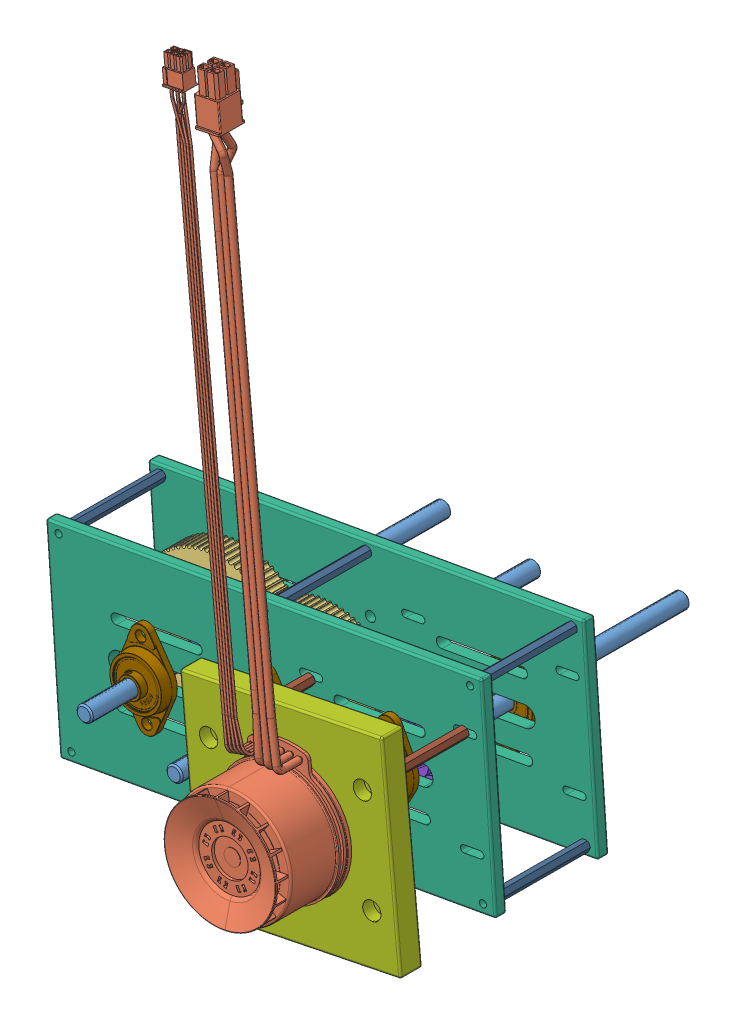
SolidWorks assembly Assembly, configuration Default. Lengths in mm.
Overall size (235.9 403.12 260.01).
25 component instances, 11 part files, 48 mates.
Components (placement in the parent):
- 1265K64_Rotary Shaft-1: 1265K64_Rotary Shaft [1265K64] at (277.2375 -256.7414 10.4805) x (-0.834942 -0.544047 0.082971) z (0.05862 0.061986 0.996354) size (8 8 200)
- 1265K64_Rotary Shaft-2: 1265K64_Rotary Shaft [1265K64] at (218.9474 -262.2229 29.581) x (0.998279 -0.00182 -0.05862) z (0.05862 0.061986 0.996354) size (8 8 200)
- 1265K64_Rotary Shaft-3: 1265K64_Rotary Shaft [1265K64] at (159.0131 -271.6943 16.4934) x (0.995771 0.067098 -0.06276) z (0.05862 0.061986 0.996354) size (8 8 200)
- EC60fl-200W-V2.stp-1: EC60fl-200W-V2.stp [Default] at (282.4403 -251.2399 98.9109) x (0.05862 0.061986 0.996354) z (0.986782 0.14745 -0.067231) size (68.19 353.93 60)
- 80 tooth pulley.stp-1: 80 tooth pulley.stp [Default] at (220.6003 -260.4751 57.675) x (0.997636 0.032205 -0.060699) z (0.05862 0.061986 0.996354) size (75.56 75.56 22.21)
- 80 tooth pulley.stp-2: 80 tooth pulley.stp [Default] at (160.6699 -269.9423 44.6536) x (0.983509 -0.174648 -0.046999) z (0.05862 0.061986 0.996354) size (75.56 75.56 22.21)
- 2463K28_Clamping Precision Flexible Shaft Coupling-1: 2463K28_Clamping Precision Flexible Shaft Coupling [2463K28] at (282.4471 -251.2327 99.0265) x (-0.5684 -0.818416 0.084358) z (0.05862 0.061986 0.996354) size (26.29 26.14 30)
- 94630A112_Steel Oversized Washer-1: 94630A112_Steel Oversized Washer [94630A112] at (219.6037 -261.5289 40.737) x (0.842889 -0.537845 -0.01613) z (0.05862 0.061986 0.996354) size (23 23 4.3)
- Shaft_and_Bearing_plate-1: Shaft_and_Bearing_plate [Default] at (221.2998 -259.7354 69.5646) x (0.99004 0.124365 -0.065986) z (0.128002 -0.990298 0.054079) size (215 6 100)
- Shaft_and_Bearing_plate-2: Shaft_and_Bearing_plate [Default] at (217.9702 -263.2563 12.9717) x (0.99004 0.124365 -0.065986) z (0.128002 -0.990298 0.054079) size (215 6 100)
- motor_plate-1: motor_plate [Default] at (283.4427 -250.1799 115.9486) x (-0.986782 -0.14745 0.067231) z (-0.151079 0.987125 -0.052524) size (100 12 100)
- 30toothpulley.stp-1: 30toothpulley.stp [Default] at (279.8164 -254.0145 54.3129) x (0.779271 0.620967 -0.084481) z (0.05862 0.061986 0.996354) size (31.8 31.8 20.6)
- 30toothpulley.stp-2: 30toothpulley.stp [Default] at (218.8358 -262.3409 27.6848) x (-0.996812 -0.050484 0.061788) z (-0.05862 -0.061986 -0.996354) size (31.8 31.8 20.6)
- KFL08 - Mancal Flange oval Ø8.stp-1: KFL08 - Mancal Flange oval Ø8.stp [Default] at (217.9702 -263.2563 12.9717) x (0.128002 -0.990298 0.054079) z (0.99004 0.124365 -0.065986) size (47.88 11.35 28.12)
- KFL08 - Mancal Flange oval Ø8.stp-2: KFL08 - Mancal Flange oval Ø8.stp [Default] at (159.0407 -271.6651 16.9619) x (0.043052 -0.997299 0.059512) z (0.997352 0.039406 -0.061131) size (47.88 11.35 28.12)
- KFL08 - Mancal Flange oval Ø8.stp-3: KFL08 - Mancal Flange oval Ø8.stp [Default] at (162.722 -267.7724 79.533) x (0.143739 -0.988194 0.053022) z (-0.987878 -0.140107 0.066838) size (47.88 11.35 28.12)
- KFL08 - Mancal Flange oval Ø8.stp-4: KFL08 - Mancal Flange oval Ø8.stp [Default] at (221.6515 -259.3635 75.5427) x (-0.128002 0.990298 -0.054079) z (0.99004 0.124365 -0.065986) size (47.88 11.35 28.12)
- KFL08 - Mancal Flange oval Ø8.stp-5: KFL08 - Mancal Flange oval Ø8.stp [Default] at (277.1557 -256.828 9.0896) x (-0.089563 0.994372 -0.056594) z (-0.994255 -0.085919 0.063842) size (47.88 11.35 28.12)
- KFL08 - Mancal Flange oval Ø8.stp-6: KFL08 - Mancal Flange oval Ø8.stp [Default] at (280.837 -252.9352 71.6606) x (-0.024433 0.99786 -0.060643) z (0.997981 0.020789 -0.06001) size (47.88 11.35 28.12)
- 91115A824_Female Threaded Hex Standoff 2in-1: 91115A824_Female Threaded Hex Standoff 2in [91115A824] at (314.4758 -203.6283 35.099) x (0.981398 0.179196 -0.068889) z (0.05862 0.061986 0.996354) size (4.76 5.5 51.24)
- 91115A824_Female Threaded Hex Standoff 2in-2: 91115A824_Female Threaded Hex Standoff 2in [91115A824] at (326.124 -293.7454 40.0202) x (-0.91308 0.40679 0.028413) z (-0.05862 -0.061986 -0.996354) size (4.76 5.5 51.24)
- 91115A824_Female Threaded Hex Standoff 2in-3: 91115A824_Female Threaded Hex Standoff 2in [91115A824] at (213.9868 -216.2513 41.7966) x (0.988326 0.136991 -0.066671) z (-0.05862 -0.061986 -0.996354) size (4.76 5.5 51.24)
- 91115A824_Female Threaded Hex Standoff 2in-4: 91115A824_Female Threaded Hex Standoff 2in [91115A824] at (113.4977 -228.8743 48.4942) x (0.263743 -0.963569 0.044429) z (-0.05862 -0.061986 -0.996354) size (4.76 5.5 51.24)
- 91115A822_Female Threaded Hex Standoff 1 and 3_4ths-1: 91115A822_Female Threaded Hex Standoff 1 and 3_4ths [91115A822] at (315.8606 -221.2764 89.9367) x (0.90677 0.414135 -0.079114) z (0.05862 0.061986 0.996354) size (4.76 5.5 44.89)
- 91115A822_Female Threaded Hex Standoff 1 and 3_4ths-2: 91115A822_Female Threaded Hex Standoff 1 and 3_4ths [91115A822] at (240.8652 -232.4825 95.0463) x (0.90677 0.414135 -0.079114) z (0.05862 0.061986 0.996354) size (4.76 5.5 44.89)
Mates (geometry in assembly coordinates):
- Concentric2: concentric aligned: cylinder of 1265K64_Rotary Shaft-2 through (224.8094 -256.0243 129.2164) axis (-0.05862 -0.061986 -0.996354) radius 4; cylinder of 80 tooth pulley.stp-1 through (221.185 -259.8568 67.6137) axis (-0.05862 -0.061986 -0.996354) radius 4
- Concentric3: concentric aligned: cylinder of 1265K64_Rotary Shaft-3 through (164.8752 -265.4956 116.1288) axis (-0.05862 -0.061986 -0.996354) radius 4; cylinder of 80 tooth pulley.stp-2 through (161.2547 -269.324 54.5922) axis (-0.05862 -0.061986 -0.996354) radius 4
- Concentric4: concentric aligned: cylinder of 1265K64_Rotary Shaft-2 through (224.8094 -256.0243 129.2164) axis (-0.05862 -0.061986 -0.996354) radius 4; cylinder of 94630A112_Steel Oversized Washer-1 through (219.8558 -261.2623 45.0213) axis (-0.05862 -0.061986 -0.996354) radius 4.2
- Concentric22: concentric aligned: cylinder of 1265K64_Rotary Shaft-2 through (224.8094 -256.0243 129.2164) axis (-0.05862 -0.061986 -0.996354) radius 4; cylinder of Shaft_and_Bearing_plate-2 through (218.3219 -262.8843 18.9498) axis (-0.05862 -0.061986 -0.996354) radius 5
- Coincident9: coincident anti-aligned: plane of 80 tooth pulley.stp-1 through (219.8558 -261.2623 45.0213) normal (-0.05862 -0.061986 -0.996354); plane of 94630A112_Steel Oversized Washer-1 through (219.8558 -261.2623 45.0213) normal (0.05862 0.061986 0.996354)
- Tangent8: tangent anti-aligned: cylinder of 1265K64_Rotary Shaft-3 through (164.8752 -265.4956 116.1288) axis (-0.05862 -0.061986 -0.996354) radius 4; plane of Shaft_and_Bearing_plate-1 through (187.6401 -268.6678 78.1226) normal (-0.128002 0.990298 -0.054079)
- Parallel3: parallel aligned: cylinder of 1265K64_Rotary Shaft-2 through (224.8094 -256.0243 129.2164) axis (-0.05862 -0.061986 -0.996354) radius 4; cylinder of 1265K64_Rotary Shaft-3 through (164.8752 -265.4956 116.1288) axis (-0.05862 -0.061986 -0.996354) radius 4
- Tangent9: tangent anti-aligned: cylinder of 1265K64_Rotary Shaft-1 through (283.0995 -250.5428 110.1159) axis (-0.05862 -0.061986 -0.996354) radius 4; plane of Shaft_and_Bearing_plate-2 through (253.6133 -263.4831 16.9107) normal (-0.128002 0.990298 -0.054079)
- Parallel4: parallel aligned: cylinder of 1265K64_Rotary Shaft-1 through (283.0995 -250.5428 110.1159) axis (-0.05862 -0.061986 -0.996354) radius 4; cylinder of 1265K64_Rotary Shaft-2 through (224.8094 -256.0243 129.2164) axis (-0.05862 -0.061986 -0.996354) radius 4
- Distance3: distance = 59.66 mm: cylinder of 1265K64_Rotary Shaft-2 through (224.8094 -256.0243 129.2164) axis (-0.05862 -0.061986 -0.996354) radius 4; cylinder of 1265K64_Rotary Shaft-1 through (283.0995 -250.5428 110.1159) axis (-0.05862 -0.061986 -0.996354) radius 4
- Distance4: distance = 59.66 mm: cylinder of 1265K64_Rotary Shaft-3 through (164.8752 -265.4956 116.1288) axis (-0.05862 -0.061986 -0.996354) radius 4; cylinder of 1265K64_Rotary Shaft-2 through (224.8094 -256.0243 129.2164) axis (-0.05862 -0.061986 -0.996354) radius 4
- Concentric34: concentric aligned: cylinder of 1265K64_Rotary Shaft-1 through (283.0995 -250.5428 110.1159) axis (-0.05862 -0.061986 -0.996354) radius 4; cylinder of motor_plate-1 through (283.7944 -249.808 121.9267) axis (-0.05862 -0.061986 -0.996354) radius 13.5
- Concentric35: concentric anti-aligned: cylinder of 1265K64_Rotary Shaft-1 through (283.0995 -250.5428 110.1159) axis (-0.05862 -0.061986 -0.996354) radius 4; cylinder of EC60fl-200W-V2.stp-1 through (282.2606 -251.4299 95.8571) axis (0.05862 0.061986 0.996354) radius 4
- Concentric36: concentric aligned: cylinder of EC60fl-200W-V2.stp-1 through (264.2888 -241.4217 130.9743) axis (-0.05862 -0.061986 -0.996354) radius 1.65; cylinder of motor_plate-1 through (263.7969 -241.9419 122.6139) axis (-0.05862 -0.061986 -0.996354) radius 2.65
- Coincident20: coincident anti-aligned: plane of EC60fl-200W-V2.stp-1 through (283.7944 -249.808 121.9267) normal (-0.05862 -0.061986 -0.996354); plane of motor_plate-1 through (283.7944 -249.808 121.9267) normal (0.05862 0.061986 0.996354)
- Concentric38: concentric anti-aligned: cylinder of EC60fl-200W-V2.stp-1 through (282.2606 -251.4299 95.8571) axis (0.05862 0.061986 0.996354) radius 4; cylinder of 2463K28_Clamping Precision Flexible Shaft Coupling-1 through (283.3264 -250.3029 113.9718) axis (-0.05862 -0.061986 -0.996354) radius 4
- Concentric44: concentric anti-aligned: cylinder of 1265K64_Rotary Shaft-1 through (283.0995 -250.5428 110.1159) axis (-0.05862 -0.061986 -0.996354) radius 4; cylinder of 30toothpulley.stp-1 through (278.3852 -255.5278 29.9882) axis (0.05862 0.061986 0.996354) radius 4
- Concentric45: concentric aligned: cylinder of 1265K64_Rotary Shaft-2 through (224.8094 -256.0243 129.2164) axis (-0.05862 -0.061986 -0.996354) radius 4; cylinder of 30toothpulley.stp-2 through (220.267 -260.8276 52.0095) axis (-0.05862 -0.061986 -0.996354) radius 4
- Coincident29: coincident anti-aligned: plane of 94630A112_Steel Oversized Washer-1 through (219.6037 -261.5289 40.737) normal (-0.05862 -0.061986 -0.996354); plane of 30toothpulley.stp-2 through (219.6037 -261.5289 40.737) normal (0.05862 0.061986 0.996354)
- Concentric46: concentric aligned: cylinder of 1265K64_Rotary Shaft-1 through (283.0995 -250.5428 110.1159) axis (-0.05862 -0.061986 -0.996354) radius 4; cylinder of KFL08 - Mancal Flange oval Ø8.stp-6 through (281.1844 -252.568 77.564) axis (-0.05862 -0.061986 -0.996354) radius 4
- Concentric47: concentric anti-aligned: cylinder of 1265K64_Rotary Shaft-1 through (283.0995 -250.5428 110.1159) axis (-0.05862 -0.061986 -0.996354) radius 4; cylinder of KFL08 - Mancal Flange oval Ø8.stp-5 through (276.8083 -257.1953 3.1862) axis (0.05862 0.061986 0.996354) radius 4
- Concentric48: concentric anti-aligned: cylinder of 1265K64_Rotary Shaft-2 through (224.8094 -256.0243 129.2164) axis (-0.05862 -0.061986 -0.996354) radius 4; cylinder of KFL08 - Mancal Flange oval Ø8.stp-1 through (217.6228 -263.6235 7.0683) axis (0.05862 0.061986 0.996354) radius 4
- Concentric49: concentric aligned: cylinder of 1265K64_Rotary Shaft-2 through (224.8094 -256.0243 129.2164) axis (-0.05862 -0.061986 -0.996354) radius 4; cylinder of KFL08 - Mancal Flange oval Ø8.stp-4 through (221.9989 -258.9962 81.4461) axis (-0.05862 -0.061986 -0.996354) radius 4
- Concentric50: concentric anti-aligned: cylinder of 1265K64_Rotary Shaft-3 through (164.8752 -265.4956 116.1288) axis (-0.05862 -0.061986 -0.996354) radius 4; cylinder of KFL08 - Mancal Flange oval Ø8.stp-2 through (158.6934 -272.0324 11.0585) axis (0.05862 0.061986 0.996354) radius 4
- Concentric51: concentric aligned: cylinder of 1265K64_Rotary Shaft-3 through (164.8752 -265.4956 116.1288) axis (-0.05862 -0.061986 -0.996354) radius 4; cylinder of KFL08 - Mancal Flange oval Ø8.stp-3 through (163.0694 -267.4051 85.4364) axis (-0.05862 -0.061986 -0.996354) radius 4
- Coincident30: coincident anti-aligned: plane of Shaft_and_Bearing_plate-1 through (221.6515 -259.3635 75.5427) normal (0.05862 0.061986 0.996354); plane of KFL08 - Mancal Flange oval Ø8.stp-3 through (176.1185 -265.8724 78.6266) normal (-0.05862 -0.061986 -0.996354)
- Coincident31: coincident anti-aligned: plane of Shaft_and_Bearing_plate-1 through (221.6515 -259.3635 75.5427) normal (0.05862 0.061986 0.996354); plane of KFL08 - Mancal Flange oval Ø8.stp-4 through (208.2258 -261.05 76.4375) normal (-0.05862 -0.061986 -0.996354)
- Coincident32: coincident anti-aligned: plane of Shaft_and_Bearing_plate-1 through (221.6515 -259.3635 75.5427) normal (0.05862 0.061986 0.996354); plane of KFL08 - Mancal Flange oval Ø8.stp-6 through (267.3036 -253.2172 72.4744) normal (-0.05862 -0.061986 -0.996354)
- Coincident33: coincident anti-aligned: plane of Shaft_and_Bearing_plate-2 through (217.9702 -263.2563 12.9717) normal (-0.05862 -0.061986 -0.996354); plane of KFL08 - Mancal Flange oval Ø8.stp-5 through (290.6386 -255.6629 8.2238) normal (0.05862 0.061986 0.996354)
- Coincident34: coincident anti-aligned: plane of Shaft_and_Bearing_plate-2 through (217.9702 -263.2563 12.9717) normal (-0.05862 -0.061986 -0.996354); plane of KFL08 - Mancal Flange oval Ø8.stp-1 through (204.5444 -264.9427 13.8665) normal (0.05862 0.061986 0.996354)
- Coincident35: coincident anti-aligned: plane of Shaft_and_Bearing_plate-2 through (217.9702 -263.2563 12.9717) normal (-0.05862 -0.061986 -0.996354); plane of KFL08 - Mancal Flange oval Ø8.stp-2 through (145.5158 -272.1995 17.7909) normal (0.05862 0.061986 0.996354)
- Concentric52: concentric anti-aligned: cylinder of Shaft_and_Bearing_plate-2 through (215.9859 -244.8114 17.9629) axis (-0.05862 -0.061986 -0.996354) radius 2.5; cylinder of KFL08 - Mancal Flange oval Ø8.stp-1 through (215.5286 -245.2949 10.1913) axis (0.05862 0.061986 0.996354) radius 2.5
- Concentric53: concentric aligned: cylinder of Shaft_and_Bearing_plate-1 through (219.3155 -241.2906 74.5558) axis (-0.05862 -0.061986 -0.996354) radius 2.5; cylinder of KFL08 - Mancal Flange oval Ø8.stp-4 through (219.421 -241.179 76.3492) axis (-0.05862 -0.061986 -0.996354) radius 2.5
- Concentric54: concentric aligned: cylinder of Shaft_and_Bearing_plate-1 through (316.3165 -201.6819 66.3845) axis (-0.05862 -0.061986 -0.996354) radius 1.75; circle of 91115A824_Female Threaded Hex Standoff 2in-1
- Coincident36: coincident anti-aligned: plane of Shaft_and_Bearing_plate-1 through (221.2998 -259.7354 69.5646) normal (-0.05862 -0.061986 -0.996354); plane of 91115A824_Female Threaded Hex Standoff 2in-1 through (315.4621 -199.3541 60.268) normal (0.05862 0.061986 0.996354)
- Concentric55: concentric aligned: cylinder of Shaft_and_Bearing_plate-2 through (312.9869 -205.2027 9.7916) axis (-0.05862 -0.061986 -0.996354) radius 1.75; circle of 91115A824_Female Threaded Hex Standoff 2in-1
- Coincident37: coincident anti-aligned: plane of Shaft_and_Bearing_plate-2 through (218.3219 -262.8843 18.9498) normal (0.05862 0.061986 0.996354); plane of 91115A824_Female Threaded Hex Standoff 2in-1 through (312.4842 -202.503 9.6533) normal (-0.05862 -0.061986 -0.996354)
- Concentric56: concentric anti-aligned: cylinder of Shaft_and_Bearing_plate-1 through (327.9647 -291.799 71.3057) axis (-0.05862 -0.061986 -0.996354) radius 1.75; circle of 91115A824_Female Threaded Hex Standoff 2in-2
- Coincident39: coincident anti-aligned: plane of Shaft_and_Bearing_plate-1 through (221.2998 -259.7354 69.5646) normal (-0.05862 -0.061986 -0.996354); plane of 91115A824_Female Threaded Hex Standoff 2in-2 through (328.7226 -289.6649 65.1064) normal (0.05862 0.061986 0.996354)
- Concentric57: concentric anti-aligned: cylinder of Shaft_and_Bearing_plate-1 through (215.8275 -214.3049 73.0821) axis (-0.05862 -0.061986 -0.996354) radius 1.75; circle of 91115A824_Female Threaded Hex Standoff 2in-3
- Coincident40: coincident anti-aligned: plane of Shaft_and_Bearing_plate-1 through (221.2998 -259.7354 69.5646) normal (-0.05862 -0.061986 -0.996354); plane of 91115A824_Female Threaded Hex Standoff 2in-3 through (215.8624 -217.3952 67.2504) normal (0.05862 0.061986 0.996354)
- Concentric58: concentric anti-aligned: cylinder of Shaft_and_Bearing_plate-1 through (115.3384 -226.928 79.7797) axis (-0.05862 -0.061986 -0.996354) radius 1.75; circle of 91115A824_Female Threaded Hex Standoff 2in-4
- Coincident41: coincident anti-aligned: plane of Shaft_and_Bearing_plate-1 through (221.2998 -259.7354 69.5646) normal (-0.05862 -0.061986 -0.996354); plane of 91115A824_Female Threaded Hex Standoff 2in-4 through (112.3393 -228.0153 74.0019) normal (0.05862 0.061986 0.996354)
- Concentric59: concentric aligned: cylinder of motor_plate-1 through (317.5152 -219.5268 118.0588) axis (-0.05862 -0.061986 -0.996354) radius 1.75; circle of 91115A822_Female Threaded Hex Standoff 1 and 3_4ths-1
- Coincident42: coincident anti-aligned: plane of motor_plate-1 through (283.4427 -250.1799 115.9486) normal (-0.05862 -0.061986 -0.996354); plane of 91115A822_Female Threaded Hex Standoff 1 and 3_4ths-1 through (316.0154 -217.4018 111.9929) normal (0.05862 0.061986 0.996354)
- Coincident43: coincident anti-aligned: plane of Shaft_and_Bearing_plate-1 through (221.6515 -259.3635 75.5427) normal (0.05862 0.061986 0.996354); plane of 91115A822_Female Threaded Hex Standoff 1 and 3_4ths-1 through (313.4097 -220.1571 67.705) normal (-0.05862 -0.061986 -0.996354)
- Concentric60: concentric aligned: cylinder of motor_plate-1 through (242.5197 -230.733 123.1684) axis (-0.05862 -0.061986 -0.996354) radius 1.75; circle of 91115A822_Female Threaded Hex Standoff 1 and 3_4ths-2
- Coincident45: coincident anti-aligned: plane of motor_plate-1 through (283.4427 -250.1799 115.9486) normal (-0.05862 -0.061986 -0.996354); plane of 91115A822_Female Threaded Hex Standoff 1 and 3_4ths-2 through (241.02 -228.6079 117.1024) normal (0.05862 0.061986 0.996354)
